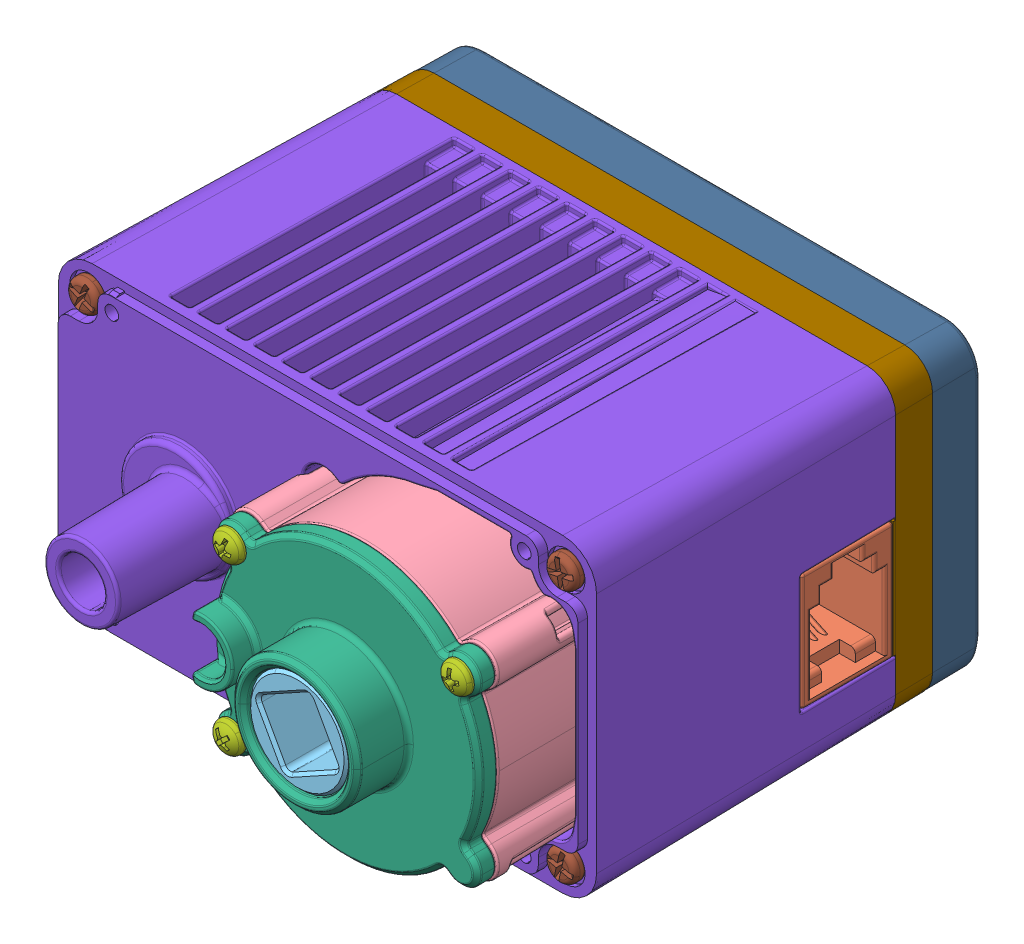
SolidWorks assembly V5 Smart Motor (276-4840) no cap, configuration Default. Lengths in mm.
Overall size (59.01 35.33 59.91).
20 component instances, 12 part files, 0 mates.
Components (placement in the parent):
- V5 Smart Motor (276-4840).step-1: V5 Smart Motor (276-4840).step [Default] at origin size (59.01 35.33 59.91)
  - 276-4840-900 Rev6_Instruction.step-1: 276-4840-900 Rev6_Instruction.step [Default] at (-14.3 0 -17.2) size (52.79 15.94 38.15)
    - 276-4840-901 Rev6.step-1: 276-4840-901 Rev6.step [Default] at (10.75 -10.05 17.8) x (-1 0 0) z (0 0 1) size (49.9 1.6 38.15)
    - 276-4840-902 Rev2.step-1: 276-4840-902 Rev2.step [Default] at (31.25 -9.25 6.2) x (0 0 -1) z (0 -1 0) size (10.35 11.39 15.94)
    - 276-4840-022 Rev4.step-1: 276-4840-022 Rev4.step [Default] at (31.25 -9.25 6.2) x (0 0 -1) z (1 0 0) size (10.26 9.1 5.51)
  - 276-4840-110 Rev10_Instruction.step-1: 276-4840-110 Rev10_Instruction.step [Default] at (12.7 0 14.7) size (35.33 35.33 31.1)
    - 276-4840-061 Rev7_Ring_Gear_Fixed01 .6 Rev3.step-1: 276-4840-061 Rev7_Ring_Gear_Fixed01 .6 Rev3.step [Default] at origin size (28.79 28.39 24.6)
    - 276-4840-018 Rev6.step-1: 276-4840-018 Rev6.step [Default] at (0 0 6.7) x (-0.483174 0.875524 0) z (0 0 1) size (26 26 12.3)
    - 276-4840-059 Rev2.step-1: 276-4840-059 Rev2.step [Default] at (0 0 10.3) size (28.4 28.4 8.5)
    - 276-4840-062 Rev1.step-1: 276-4840-062 Rev1.step [Default] at (-12.1353 8.8168 12.3) x (0.956835 -0.290632 0) z (-0.290632 -0.956835 0) size (3.2 6.56 3.2)
    - 276-4840-062 Rev1.step-2: 276-4840-062 Rev1.step [Default] at (12.1353 8.8168 12.3) x (0.978427 0.206591 0) z (0.206591 -0.978427 0) size (3.2 6.56 3.2)
    - 276-4840-062 Rev1.step-3: 276-4840-062 Rev1.step [Default] at (-12.1353 -8.8168 12.3) x (0.72563 0.688086 0) z (0.688086 -0.72563 0) size (3.2 6.56 3.2)
  - 276-4840-001 Rev38.step-1: 276-4840-001 Rev38.step [Default] at origin size (57.3 33 46.9)
  - 276-4840-005 Rev27.step-1: 276-4840-005 Rev27.step [Default] at (0 0 -17.95) size (56.17 31.87 12.9)
  - 276-4840-004 Rev16.step-1: 276-4840-004 Rev16.step [Default] at (0 0 -19.2) size (56.01 31.71 9.21)
  - 276-4840-009 Rev3.step-1: 276-4840-009 Rev3.step [Default] at (25.45 13.5 15.7) x (0.19987 -0.979823 0) z (-0.979823 -0.19987 0) size (3.4 41.31 4.34)
  - 276-4840-009 Rev3.step-2: 276-4840-009 Rev3.step [Default] at (-25.45 -13.5 15.7) x (-0.998855 0.047836 0) z (0.047836 0.998855 0) size (3.4 41.31 4.34)
  - 276-4840-009 Rev3.step-3: 276-4840-009 Rev3.step [Default] at (25.45 -13.5 15.7) x (-0.975374 0.220559 0) z (0.220559 0.975374 0) size (3.4 41.31 4.34)
  - 276-4840-009 Rev3.step-4: 276-4840-009 Rev3.step [Default] at (-25.45 13.5 15.7) x (-0.922256 0.38658 0) z (0.38658 0.922256 0) size (3.4 41.31 4.34)
  - 276-4840-025 Rev19.step-1: 276-4840-025 Rev19.step [Default] at (12.7 0 -22.63) x (-0.993315 0.115437 0) z (0 0 1) size (14.82 14.83 35.18)
